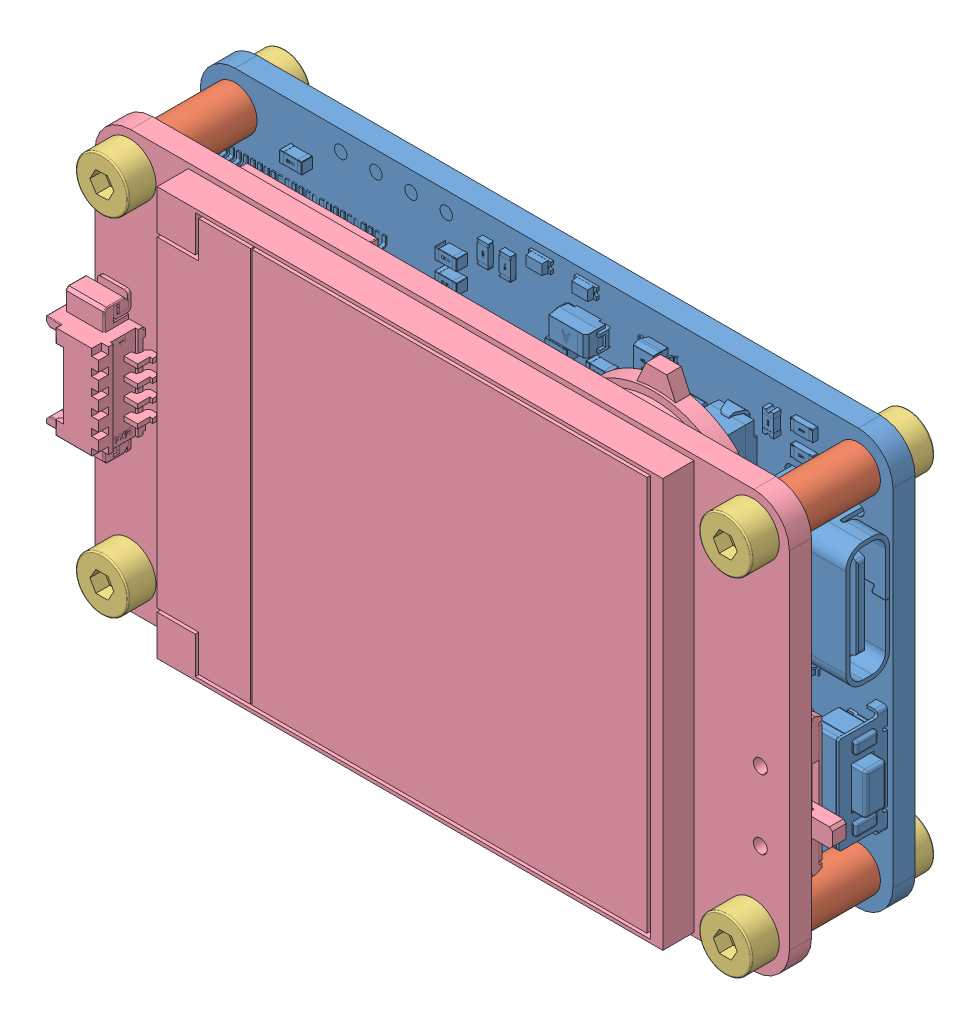
SolidWorks assembly 整合体, configuration 默认. Lengths in mm.
Overall size (51.92 32.2 14.6).
14 component instances, 4 part files, 11 mates.
Components (placement in the parent):
- STM32H7_Core-1: STM32H7_Core [默认] at (-0.3844 0.6819 49.011) size (50.62 30.64 6.26)
- M2铜柱-1: M2铜柱 [默认] at (22.1156 -11.8181 55.011) x (-0.923728 -0.383049 0) z (0 0 -1) size (3.2 3.2 6)
- M2铜柱-2: M2铜柱 [默认] at (-22.8844 -11.8181 49.011) size (3.2 3.2 6)
- M2铜柱-3: M2铜柱 [默认] at (-22.8844 13.1819 55.011) x (-0.923728 -0.383049 0) z (0 0 -1) size (3.2 3.2 6)
- M2铜柱-4: M2铜柱 [默认] at (22.1156 13.1819 55.011) x (-0.923728 -0.383049 0) z (0 0 -1) size (3.2 3.2 6)
- 内六角圆柱头螺钉M2-1: 内六角圆柱头螺钉M2 [M2×3] at (-22.8844 -11.8181 45.411) x (0 0 1) z (-0.457721 0.889096 0) size (5 3.8 3.8)
- 内六角圆柱头螺钉M2-2: 内六角圆柱头螺钉M2 [M2×3] at (22.1156 -11.8181 58.611) x (0 0 -1) z (1 0 0) size (5 3.8 3.8)
- 内六角圆柱头螺钉M2-3: 内六角圆柱头螺钉M2 [M2×3] at (-22.8844 13.1819 58.611) x (0 0 -1) z (0.999089 0.042672 0) size (5 3.8 3.8)
- 内六角圆柱头螺钉M2-4: 内六角圆柱头螺钉M2 [M2×3] at (-22.8844 13.1819 45.411) x (0 0 1) z (-0.923728 -0.383049 0) size (5 3.8 3.8)
- 内六角圆柱头螺钉M2-5: 内六角圆柱头螺钉M2 [M2×3] at (22.1156 13.1819 58.611) x (0 0 -1) z (1 0 0) size (5 3.8 3.8)
- 内六角圆柱头螺钉M2-6: 内六角圆柱头螺钉M2 [M2×3] at (22.1156 -11.8181 45.411) x (0 0 1) z (-0.923728 -0.383049 0) size (5 3.8 3.8)
- 内六角圆柱头螺钉M2-7: 内六角圆柱头螺钉M2 [M2×3] at (-22.8844 -11.8181 58.611) x (0 0 -1) z (1 0 0) size (5 3.8 3.8)
- 内六角圆柱头螺钉M2-8: 内六角圆柱头螺钉M2 [M2×3] at (22.1156 13.1819 45.411) x (0 0 1) z (-0.923728 -0.383049 0) size (5 3.8 3.8)
- STM32H7_Expand-2: STM32H7_Expand [默认] at (-0.3204 0.6179 56.611) size (51.92 31.7 8.21)
Mates (geometry in assembly coordinates):
- 重合12: coincident anti-aligned: circle of STM32H7_Core-1; circle of M2铜柱-3
- 重合13: coincident anti-aligned: circle of STM32H7_Core-1; circle of M2铜柱-4
- 重合14: coincident aligned: circle of STM32H7_Core-1; circle of M2铜柱-2
- 重合15: coincident anti-aligned: circle of STM32H7_Core-1; circle of M2铜柱-1
- 重合22: coincident aligned: circle of STM32H7_Core-1; circle of 内六角圆柱头螺钉M2-8
- 重合23: coincident aligned: circle of STM32H7_Core-1; circle of 内六角圆柱头螺钉M2-6
- 重合24: coincident aligned: circle of STM32H7_Core-1; circle of 内六角圆柱头螺钉M2-4
- 重合25: coincident aligned: circle of STM32H7_Core-1; circle of 内六角圆柱头螺钉M2-1
- 重合26: coincident anti-aligned: plane of M2铜柱-3 through (-22.8844 13.1819 55.011) normal (0 0 1); plane of STM32H7_Expand-2 through (-25.3844 -11.8821 55.011) normal (0 0 -1)
- 重合27: coincident aligned: plane of STM32H7_Core-1 through (-22.8844 15.6819 47.411) normal (0 1 0); plane of STM32H7_Expand-2 through (-22.8204 15.6819 55.011) normal (0 1 0)
- 重合28: coincident aligned: plane of STM32H7_Core-1 through (-25.3844 -11.8181 47.411) normal (-1 0 0); plane of STM32H7_Expand-2 through (-25.3844 -11.8821 55.011) normal (-1 0 0)
